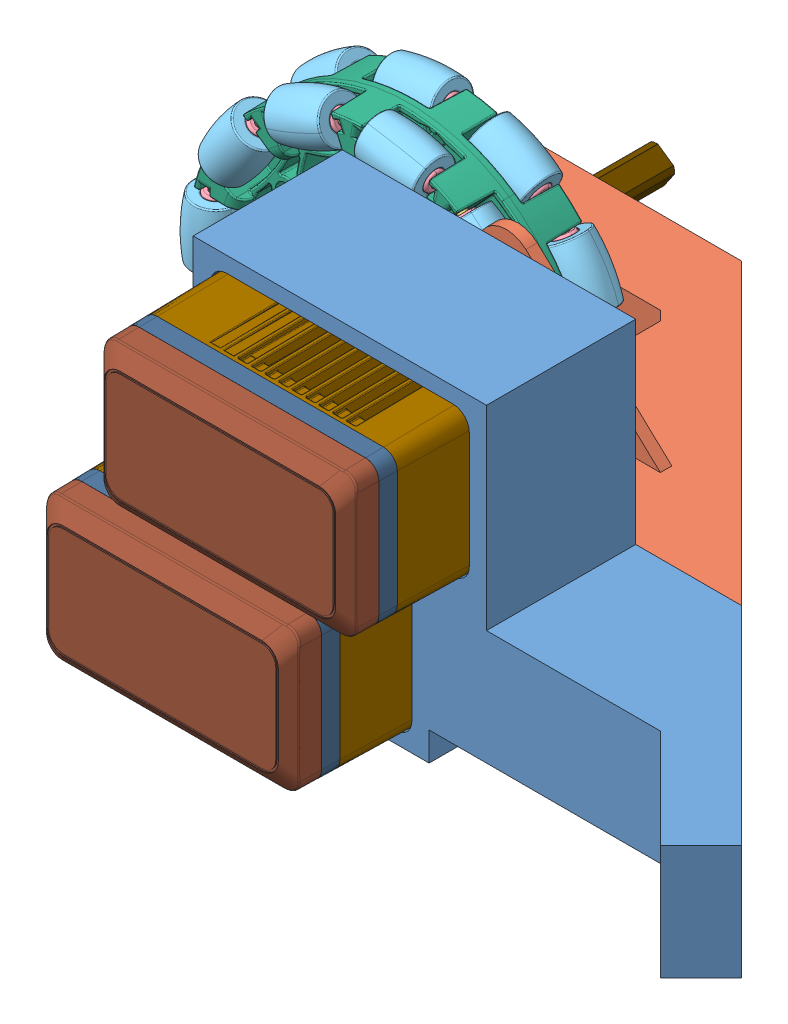
SolidWorks assembly Assem1, configuration Default. Lengths in mm.
Overall size (215.08 121.96 147.68).
139 component instances, 24 part files, 28 mates.
Components (placement in the parent):
- MotorBracket1-1: MotorBracket1 [Default] at (44.7562 139.8317 99.5148) size (165.36 74.93 54.97)
- V5 Smart Motor (276-4840) no cap 2-1: V5 Smart Motor (276-4840) no cap 2 [Default] at (82.8562 152.5317 238.3808) x (-1 0 0) z (0 0 -1) size (59.01 35.33 59.91)
  - 276-4840-900 Rev6_Instruction.step-1: 276-4840-900 Rev6_Instruction.step [Default] at (-14.3 0 -17.2) size (52.79 15.94 38.15)
    - 276-4840-901 Rev6.step-1: 276-4840-901 Rev6.step [Default] at (10.75 -10.05 17.8) x (-1 0 0) z (0 0 1) size (49.9 1.6 38.15)
    - 276-4840-902 Rev2.step-1: 276-4840-902 Rev2.step [Default] at (31.25 -9.25 6.2) x (0 0 -1) z (0 -1 0) size (10.35 11.39 15.94)
    - 276-4840-022 Rev4.step-1: 276-4840-022 Rev4.step [Default] at (31.25 -9.25 6.2) x (0 0 -1) z (1 0 0) size (10.26 9.1 5.51)
  - 276-4840-110 Rev10_Instruction.step-1: 276-4840-110 Rev10_Instruction.step [Default] at (12.7 0 14.7) size (35.33 35.33 31.1)
    - 276-4840-061 Rev7_Ring_Gear_Fixed01 .6 Rev3.step-1: 276-4840-061 Rev7_Ring_Gear_Fixed01 .6 Rev3.step [Default] at origin size (28.79 28.39 24.6)
    - 276-4840-018 Rev6.step-1: 276-4840-018 Rev6.step [Default] at (0 0 6.7) x (-0.483174 0.875524 0) z (0 0 1) size (26 26 12.3)
    - 276-4840-059 Rev2.step-1: 276-4840-059 Rev2.step [Default] at (0 0 10.3) size (28.4 28.4 8.5)
    - 276-4840-062 Rev1.step-1: 276-4840-062 Rev1.step [Default] at (-12.1353 8.8168 12.3) x (0.956835 -0.290632 0) z (-0.290632 -0.956835 0) size (3.2 6.56 3.2)
    - 276-4840-062 Rev1.step-2: 276-4840-062 Rev1.step [Default] at (12.1353 8.8168 12.3) x (0.978427 0.206591 0) z (0.206591 -0.978427 0) size (3.2 6.56 3.2)
    - 276-4840-062 Rev1.step-3: 276-4840-062 Rev1.step [Default] at (-12.1353 -8.8168 12.3) x (0.72563 0.688086 0) z (0.688086 -0.72563 0) size (3.2 6.56 3.2)
  - 276-4840-001 Rev38.step-1: 276-4840-001 Rev38.step [Default] at origin size (57.3 33 46.9)
  - 276-4840-005 Rev27.step-1: 276-4840-005 Rev27.step [Default] at (0 0 -17.95) size (56.17 31.87 12.9)
  - 276-4840-004 Rev16.step-1: 276-4840-004 Rev16.step [Default] at (0 0 -19.2) size (56.01 31.71 9.21)
  - 276-4840-009 Rev3.step-1: 276-4840-009 Rev3.step [Default] at (25.45 13.5 15.7) x (0.19987 -0.979823 0) z (-0.979823 -0.19987 0) size (3.4 41.31 4.34)
  - 276-4840-009 Rev3.step-2: 276-4840-009 Rev3.step [Default] at (-25.45 -13.5 15.7) x (-0.998855 0.047836 0) z (0.047836 0.998855 0) size (3.4 41.31 4.34)
  - 276-4840-009 Rev3.step-3: 276-4840-009 Rev3.step [Default] at (25.45 -13.5 15.7) x (-0.975374 0.220559 0) z (0.220559 0.975374 0) size (3.4 41.31 4.34)
  - 276-4840-009 Rev3.step-4: 276-4840-009 Rev3.step [Default] at (-25.45 13.5 15.7) x (-0.922256 0.38658 0) z (0.38658 0.922256 0) size (3.4 41.31 4.34)
  - 276-4840-025 Rev19.step-1: 276-4840-025 Rev19.step [Default] at (12.7 0 -22.63) x (-0.993315 0.115437 0) z (0 0 1) size (14.82 14.83 35.18)
- V5 Smart Motor (276-4840) no cap 2-2: V5 Smart Motor (276-4840) no cap 2 [Default] at (95.5562 188.4527 238.3808) x (-1 0 0) z (0 0 -1) size (59.01 35.33 59.91)
  - 276-4840-900 Rev6_Instruction.step-1: 276-4840-900 Rev6_Instruction.step [Default] at (-14.3 0 -17.2) size (52.79 15.94 38.15)
    - 276-4840-901 Rev6.step-1: 276-4840-901 Rev6.step [Default] at (10.75 -10.05 17.8) x (-1 0 0) z (0 0 1) size (49.9 1.6 38.15)
    - 276-4840-902 Rev2.step-1: 276-4840-902 Rev2.step [Default] at (31.25 -9.25 6.2) x (0 0 -1) z (0 -1 0) size (10.35 11.39 15.94)
    - 276-4840-022 Rev4.step-1: 276-4840-022 Rev4.step [Default] at (31.25 -9.25 6.2) x (0 0 -1) z (1 0 0) size (10.26 9.1 5.51)
  - 276-4840-110 Rev10_Instruction.step-1: 276-4840-110 Rev10_Instruction.step [Default] at (12.7 0 14.7) size (35.33 35.33 31.1)
    - 276-4840-061 Rev7_Ring_Gear_Fixed01 .6 Rev3.step-1: 276-4840-061 Rev7_Ring_Gear_Fixed01 .6 Rev3.step [Default] at origin size (28.79 28.39 24.6)
    - 276-4840-018 Rev6.step-1: 276-4840-018 Rev6.step [Default] at (0 0 6.7) x (-0.483174 0.875524 0) z (0 0 1) size (26 26 12.3)
    - 276-4840-059 Rev2.step-1: 276-4840-059 Rev2.step [Default] at (0 0 10.3) size (28.4 28.4 8.5)
    - 276-4840-062 Rev1.step-1: 276-4840-062 Rev1.step [Default] at (-12.1353 8.8168 12.3) x (0.956835 -0.290632 0) z (-0.290632 -0.956835 0) size (3.2 6.56 3.2)
    - 276-4840-062 Rev1.step-2: 276-4840-062 Rev1.step [Default] at (12.1353 8.8168 12.3) x (0.978427 0.206591 0) z (0.206591 -0.978427 0) size (3.2 6.56 3.2)
    - 276-4840-062 Rev1.step-3: 276-4840-062 Rev1.step [Default] at (-12.1353 -8.8168 12.3) x (0.72563 0.688086 0) z (0.688086 -0.72563 0) size (3.2 6.56 3.2)
  - 276-4840-001 Rev38.step-1: 276-4840-001 Rev38.step [Default] at origin size (57.3 33 46.9)
  - 276-4840-005 Rev27.step-1: 276-4840-005 Rev27.step [Default] at (0 0 -17.95) size (56.17 31.87 12.9)
  - 276-4840-004 Rev16.step-1: 276-4840-004 Rev16.step [Default] at (0 0 -19.2) size (56.01 31.71 9.21)
  - 276-4840-009 Rev3.step-1: 276-4840-009 Rev3.step [Default] at (25.45 13.5 15.7) x (0.19987 -0.979823 0) z (-0.979823 -0.19987 0) size (3.4 41.31 4.34)
  - 276-4840-009 Rev3.step-2: 276-4840-009 Rev3.step [Default] at (-25.45 -13.5 15.7) x (-0.998855 0.047836 0) z (0.047836 0.998855 0) size (3.4 41.31 4.34)
  - 276-4840-009 Rev3.step-3: 276-4840-009 Rev3.step [Default] at (25.45 -13.5 15.7) x (-0.975374 0.220559 0) z (0.220559 0.975374 0) size (3.4 41.31 4.34)
  - 276-4840-009 Rev3.step-4: 276-4840-009 Rev3.step [Default] at (-25.45 13.5 15.7) x (-0.922256 0.38658 0) z (0.38658 0.922256 0) size (3.4 41.31 4.34)
  - 276-4840-025 Rev19.step-1: 276-4840-025 Rev19.step [Default] at (12.7 0 -22.63) x (-0.993315 0.115437 0) z (0 0 1) size (14.82 14.83 35.18)
- 0.375_ ID x 0.875_ OD x 0.281_ WD (Radial Bearing) (217-3239)-1: 0.375_ ID x 0.875_ OD x 0.281_ WD (Radial Bearing) (217-3239) [Default] at (44.7562 152.5317 213.3576) x (0 0 -1) z (1 0 0) size (7.14 22.23 22.23)
- 0.375IDtoHSshaftInsert-1: 0.375IDtoHSshaftInsert [Default] at (44.7562 152.5317 213.3576) x (0.567741 0.823207 0) z (0 0 -1) size (9.53 9.53 5.54)
- 12T High Strength Metal Pinion with HS hole (276-2251)-1: 12T High Strength Metal Pinion with HS hole (276-2251) [Default] at (44.7562 152.5317 196.9048) x (0.567741 0.823207 0) z (0.823207 -0.567741 0) size (14.8 12.7 14.8)
- 36T Gear (276-2169-002).step-1: 36T Gear (276-2169-002).step [Default] at (70.1562 152.5317 194.4473) x (0.963194 -0.268806 0) z (0 0 1) size (40.08 40.08 9.53)
- 3.75_ High Strength Shaft (276-3524)-1: 3.75_ High Strength Shaft (276-3524) [Default] at (44.7562 152.5317 213.3576) x (-0.567741 -0.823207 0) z (0 0 -1) size (6.37 6.36 95.25)
- Holo_Motor_Shaft-1: Holo_Motor_Shaft [Default] at (70.1454 152.569 338.5008) x (0.875524 -0.483174 0) z (0 0 1) size (3.28 3.28 30.48)
- WheelBracket1-1: WheelBracket1 [Default] at (44.7562 139.8317 99.5148) size (119.38 54.97 66.04)
- 3.25_ Omni-Directional Wheel (276-3526) part-1: 3.25_ Omni-Directional Wheel (276-3526) part [Default] at (44.7562 152.5317 173.2048) x (0.567741 0.823207 0) z (0 0 1) size (90.82 89.11 34)
  - 3.25_ Omni-Directional Wheel (276-3526) .step-1: 3.25_ Omni-Directional Wheel (276-3526) .step [Default] at origin size (90.82 89.11 34)
    - Roller Assembly.step-1: Roller Assembly.step [Default] at (-0.0014 35.9575 7.1) x (0 0.963098 -0.269151) z (-1 0 0) size (14.05 14.05 18.75)
      - 276-3526-001 Rev 1.step-1: 276-3526-001 Rev 1.step [Default] at origin size (2 2 18.75)
      - 276-3526-003 Rev 1.step-1: 276-3526-003 Rev 1.step [Default] at origin size (6.15 6.15 14.2)
      - 276-3526-002 Rev 1.step-1: 276-3526-002 Rev 1.step [Default] x (0 0 1) z (-0.908956 0.416893 0) size (13.2 10.6 10.6)
    - Roller Assembly.step-2: Roller Assembly.step [Default] at (-19.4287 30.2567 7.1) x (0.421057 -0.655178 0.627258) z (-0.841254 -0.540641 0) size (14.05 14.05 18.75)
      - 276-3526-001 Rev 1.step-1: 276-3526-001 Rev 1.step [Default] at origin size (2 2 18.75)
      - 276-3526-003 Rev 1.step-1: 276-3526-003 Rev 1.step [Default] at origin size (6.15 6.15 14.2)
      - 276-3526-002 Rev 1.step-1: 276-3526-002 Rev 1.step [Default] x (0 0 1) z (-0.908956 0.416893 0) size (13.2 10.6 10.6)
    - Roller Assembly.step-3: Roller Assembly.step [Default] at (-35.5935 -5.1038 7.1) x (0.979746 0.140866 -0.142315) z (0.142315 -0.989821 0) size (14.05 14.05 18.75)
      - 276-3526-001 Rev 1.step-1: 276-3526-001 Rev 1.step [Default] at origin size (2 2 18.75)
      - 276-3526-003 Rev 1.step-1: 276-3526-003 Rev 1.step [Default] at origin size (6.15 6.15 14.2)
      - 276-3526-002 Rev 1.step-1: 276-3526-002 Rev 1.step [Default] x (0 0 1) z (-0.908956 0.416893 0) size (13.2 10.6 10.6)
    - Roller Assembly.step-4: Roller Assembly.step [Default] at (-10.1434 -34.4972 7.1) x (0.079373 0.27032 -0.959493) z (0.959493 -0.281733 0) size (14.05 14.05 18.75)
      - 276-3526-001 Rev 1.step-1: 276-3526-001 Rev 1.step [Default] at origin size (2 2 18.75)
      - 276-3526-003 Rev 1.step-1: 276-3526-003 Rev 1.step [Default] at origin size (6.15 6.15 14.2)
      - 276-3526-002 Rev 1.step-1: 276-3526-002 Rev 1.step [Default] x (0 0 1) z (-0.908956 0.416893 0) size (13.2 10.6 10.6)
    - Roller Assembly.step-5: Roller Assembly.step [Default] at (27.166 -23.5574 7.1) x (-0.355209 0.30779 -0.882662) z (0.654861 0.75575 0) size (14.05 14.05 18.75)
      - 276-3526-001 Rev 1.step-1: 276-3526-001 Rev 1.step [Default] at origin size (2 2 18.75)
      - 276-3526-003 Rev 1.step-1: 276-3526-003 Rev 1.step [Default] at origin size (6.15 6.15 14.2)
      - 276-3526-002 Rev 1.step-1: 276-3526-002 Rev 1.step [Default] x (0 0 1) z (-0.908956 0.416893 0) size (13.2 10.6 10.6)
    - Roller Assembly.step-6: Roller Assembly.step [Default] at (32.7138 14.9249 7.1) x (0.89908 0.410596 0.151875) z (-0.415415 0.909632 0) size (14.05 14.05 18.75)
      - 276-3526-001 Rev 1.step-1: 276-3526-001 Rev 1.step [Default] at origin size (2 2 18.75)
      - 276-3526-003 Rev 1.step-1: 276-3526-003 Rev 1.step [Default] at origin size (6.15 6.15 14.2)
      - 276-3526-002 Rev 1.step-1: 276-3526-002 Rev 1.step [Default] x (0 0 1) z (-0.908956 0.416893 0) size (13.2 10.6 10.6)
    - Roller Assembly.step-7: Roller Assembly.step [Default] at (19.4515 30.242 7.1) x (0.194707 0.302971 0.932898) z (-0.841254 0.540641 0) size (14.05 14.05 18.75)
      - 276-3526-001 Rev 1.step-1: 276-3526-001 Rev 1.step [Default] at origin size (2 2 18.75)
      - 276-3526-003 Rev 1.step-1: 276-3526-003 Rev 1.step [Default] at origin size (6.15 6.15 14.2)
      - 276-3526-002 Rev 1.step-1: 276-3526-002 Rev 1.step [Default] x (0 0 1) z (-0.908956 0.416893 0) size (13.2 10.6 10.6)
    - Roller Assembly.step-8: Roller Assembly.step [Default] at (-32.7025 14.9497 7.1) x (0.82743 -0.377875 0.415415) z (-0.415415 -0.909632 0) size (14.05 14.05 18.75)
      - 276-3526-001 Rev 1.step-1: 276-3526-001 Rev 1.step [Default] at origin size (2 2 18.75)
      - 276-3526-003 Rev 1.step-1: 276-3526-003 Rev 1.step [Default] at origin size (6.15 6.15 14.2)
      - 276-3526-002 Rev 1.step-1: 276-3526-002 Rev 1.step [Default] x (0 0 1) z (-0.908956 0.416893 0) size (13.2 10.6 10.6)
    - Roller Assembly.step-9: Roller Assembly.step [Default] at (-27.1838 -23.5369 7.1) x (0.578931 0.501646 -0.642799) z (0.654861 -0.75575 0) size (14.05 14.05 18.75)
      - 276-3526-001 Rev 1.step-1: 276-3526-001 Rev 1.step [Default] at origin size (2 2 18.75)
      - 276-3526-003 Rev 1.step-1: 276-3526-003 Rev 1.step [Default] at origin size (6.15 6.15 14.2)
      - 276-3526-002 Rev 1.step-1: 276-3526-002 Rev 1.step [Default] x (0 0 1) z (-0.908956 0.416893 0) size (13.2 10.6 10.6)
    - Roller Assembly.step-10: Roller Assembly.step [Default] at (10.1174 -34.5048 7.1) x (0.079373 -0.27032 -0.959493) z (0.959493 0.281733 0) size (14.05 14.05 18.75)
      - 276-3526-001 Rev 1.step-1: 276-3526-001 Rev 1.step [Default] at origin size (2 2 18.75)
      - 276-3526-003 Rev 1.step-1: 276-3526-003 Rev 1.step [Default] at origin size (6.15 6.15 14.2)
      - 276-3526-002 Rev 1.step-1: 276-3526-002 Rev 1.step [Default] x (0 0 1) z (-0.908956 0.416893 0) size (13.2 10.6 10.6)
    - Roller Assembly.step-11: Roller Assembly.step [Default] at (35.5896 -5.1307 7.1) x (0.988515 -0.142127 -0.05136) z (0.142315 0.989821 0) size (14.05 14.05 18.75)
      - 276-3526-001 Rev 1.step-1: 276-3526-001 Rev 1.step [Default] at origin size (2 2 18.75)
      - 276-3526-003 Rev 1.step-1: 276-3526-003 Rev 1.step [Default] at origin size (6.15 6.15 14.2)
      - 276-3526-002 Rev 1.step-1: 276-3526-002 Rev 1.step [Default] x (0 0 1) z (-0.908956 0.416893 0) size (13.2 10.6 10.6)
    - Roller Assembly.step-12: Roller Assembly.step [Default] at (10.1434 34.4972 -7.1) x (0.083119 0.283078 -0.955489) z (0.959493 -0.281733 0) size (14.05 14.05 18.75)
      - 276-3526-001 Rev 1.step-1: 276-3526-001 Rev 1.step [Default] at origin size (2 2 18.75)
      - 276-3526-003 Rev 1.step-1: 276-3526-003 Rev 1.step [Default] at origin size (6.15 6.15 14.2)
      - 276-3526-002 Rev 1.step-1: 276-3526-002 Rev 1.step [Default] x (0 0 1) z (-0.908956 0.416893 0) size (13.2 10.6 10.6)
    - Roller Assembly.step-13: Roller Assembly.step [Default] at (27.1838 23.5369 -7.1) x (0.582526 0.504762 -0.637086) z (0.654861 -0.75575 0) size (14.05 14.05 18.75)
      - 276-3526-001 Rev 1.step-1: 276-3526-001 Rev 1.step [Default] at origin size (2 2 18.75)
      - 276-3526-003 Rev 1.step-1: 276-3526-003 Rev 1.step [Default] at origin size (6.15 6.15 14.2)
      - 276-3526-002 Rev 1.step-1: 276-3526-002 Rev 1.step [Default] x (0 0 1) z (-0.908956 0.416893 0) size (13.2 10.6 10.6)
    - Roller Assembly.step-14: Roller Assembly.step [Default] at (35.5935 5.1038 -7.1) x (0.926341 0.133188 -0.352355) z (0.142315 -0.989821 0) size (14.05 14.05 18.75)
      - 276-3526-001 Rev 1.step-1: 276-3526-001 Rev 1.step [Default] at origin size (2 2 18.75)
      - 276-3526-003 Rev 1.step-1: 276-3526-003 Rev 1.step [Default] at origin size (6.15 6.15 14.2)
      - 276-3526-002 Rev 1.step-1: 276-3526-002 Rev 1.step [Default] x (0 0 1) z (-0.908956 0.416893 0) size (13.2 10.6 10.6)
    - Roller Assembly.step-15: Roller Assembly.step [Default] at (32.7025 -14.9497 -7.1) x (0.897398 -0.409828 0.163453) z (-0.415415 -0.909632 0) size (14.05 14.05 18.75)
      - 276-3526-001 Rev 1.step-1: 276-3526-001 Rev 1.step [Default] at origin size (2 2 18.75)
      - 276-3526-003 Rev 1.step-1: 276-3526-003 Rev 1.step [Default] at origin size (6.15 6.15 14.2)
      - 276-3526-002 Rev 1.step-1: 276-3526-002 Rev 1.step [Default] x (0 0 1) z (-0.908956 0.416893 0) size (13.2 10.6 10.6)
    - Roller Assembly.step-16: Roller Assembly.step [Default] at (19.4287 -30.2567 -7.1) x (0.277612 -0.431972 0.858098) z (-0.841254 -0.540641 0) size (14.05 14.05 18.75)
      - 276-3526-001 Rev 1.step-1: 276-3526-001 Rev 1.step [Default] at origin size (2 2 18.75)
      - 276-3526-003 Rev 1.step-1: 276-3526-003 Rev 1.step [Default] at origin size (6.15 6.15 14.2)
      - 276-3526-002 Rev 1.step-1: 276-3526-002 Rev 1.step [Default] x (0 0 1) z (-0.908956 0.416893 0) size (13.2 10.6 10.6)
    - Roller Assembly.step-17: Roller Assembly.step [Default] at (-0.0136 -35.9575 -7.1) x (0 -0.239919 0.970793) z (-1 0 0) size (14.05 14.05 18.75)
      - 276-3526-001 Rev 1.step-1: 276-3526-001 Rev 1.step [Default] at origin size (2 2 18.75)
      - 276-3526-003 Rev 1.step-1: 276-3526-003 Rev 1.step [Default] at origin size (6.15 6.15 14.2)
      - 276-3526-002 Rev 1.step-1: 276-3526-002 Rev 1.step [Default] x (0 0 1) z (-0.908956 0.416893 0) size (13.2 10.6 10.6)
    - Roller Assembly.step-18: Roller Assembly.step [Default] at (-19.4515 -30.242 -7.1) x (0.31008 0.482494 0.819176) z (-0.841254 0.540641 0) size (14.05 14.05 18.75)
      - 276-3526-001 Rev 1.step-1: 276-3526-001 Rev 1.step [Default] at origin size (2 2 18.75)
      - 276-3526-003 Rev 1.step-1: 276-3526-003 Rev 1.step [Default] at origin size (6.15 6.15 14.2)
      - 276-3526-002 Rev 1.step-1: 276-3526-002 Rev 1.step [Default] x (0 0 1) z (-0.908956 0.416893 0) size (13.2 10.6 10.6)
    - Roller Assembly.step-19: Roller Assembly.step [Default] at (-32.7138 -14.9249 -7.1) x (0.58758 0.268339 0.763377) z (-0.415415 0.909632 0) size (14.05 14.05 18.75)
      - 276-3526-001 Rev 1.step-1: 276-3526-001 Rev 1.step [Default] at origin size (2 2 18.75)
      - 276-3526-003 Rev 1.step-1: 276-3526-003 Rev 1.step [Default] at origin size (6.15 6.15 14.2)
      - 276-3526-002 Rev 1.step-1: 276-3526-002 Rev 1.step [Default] x (0 0 1) z (-0.908956 0.416893 0) size (13.2 10.6 10.6)
    - Roller Assembly.step-20: Roller Assembly.step [Default] at (-35.5896 5.1307 -7.1) x (0.965498 -0.138818 0.220323) z (0.142315 0.989821 0) size (14.05 14.05 18.75)
      - 276-3526-001 Rev 1.step-1: 276-3526-001 Rev 1.step [Default] at origin size (2 2 18.75)
      - 276-3526-003 Rev 1.step-1: 276-3526-003 Rev 1.step [Default] at origin size (6.15 6.15 14.2)
      - 276-3526-002 Rev 1.step-1: 276-3526-002 Rev 1.step [Default] x (0 0 1) z (-0.908956 0.416893 0) size (13.2 10.6 10.6)
    - Roller Assembly.step-21: Roller Assembly.step [Default] at (-27.166 23.5574 -7.1) x (0.75327 -0.652712 -0.080935) z (0.654861 0.75575 0) size (14.05 14.05 18.75)
      - 276-3526-001 Rev 1.step-1: 276-3526-001 Rev 1.step [Default] at origin size (2 2 18.75)
      - 276-3526-003 Rev 1.step-1: 276-3526-003 Rev 1.step [Default] at origin size (6.15 6.15 14.2)
      - 276-3526-002 Rev 1.step-1: 276-3526-002 Rev 1.step [Default] x (0 0 1) z (-0.908956 0.416893 0) size (13.2 10.6 10.6)
    - Roller Assembly.step-22: Roller Assembly.step [Default] at (-10.1174 34.5048 -7.1) x (0.123782 -0.421563 -0.898311) z (0.959493 0.281733 0) size (14.05 14.05 18.75)
      - 276-3526-001 Rev 1.step-1: 276-3526-001 Rev 1.step [Default] at origin size (2 2 18.75)
      - 276-3526-003 Rev 1.step-1: 276-3526-003 Rev 1.step [Default] at origin size (6.15 6.15 14.2)
      - 276-3526-002 Rev 1.step-1: 276-3526-002 Rev 1.step [Default] x (0 0 1) z (-0.908956 0.416893 0) size (13.2 10.6 10.6)
    - 276-3526-004 Rev 1.step-1: 276-3526-004 Rev 1.step [Default] at origin size (78.5 78.5 19.07)
Mates (geometry in assembly coordinates):
- Coincident1: coincident anti-aligned: plane of MotorBracket1-1 through (57.8062 165.4317 221.1808) normal (0 0 1); plane of V5 Smart Motor (276-4840) no cap 2-1/276-4840-001 Rev38.step-1 through (107.9062 165.4317 221.1808) normal (0 0 -1)
- Concentric1: concentric aligned: cylinder of MotorBracket1-1 through (107.9062 165.4317 221.1808) axis (0 0 1) radius 3.6; cone of V5 Smart Motor (276-4840) no cap 2-1/276-4840-001 Rev38.step-1 through (107.9062 165.4317 222.1808) axis (0 0 1)
- Concentric2: concentric aligned: cylinder of MotorBracket1-1 through (107.9062 139.6317 221.1808) axis (0 0 1) radius 3.6; cone of V5 Smart Motor (276-4840) no cap 2-1/276-4840-001 Rev38.step-1 through (107.9062 139.6317 222.1808) axis (0 0 1)
- Concentric4: concentric aligned: cylinder of MotorBracket1-1 through (120.6062 201.3527 221.1808) axis (0 0 1) radius 3.6; cone of V5 Smart Motor (276-4840) no cap 2-2/276-4840-001 Rev38.step-1 through (120.6062 201.3527 222.1808) axis (0 0 1)
- Concentric5: concentric aligned: cylinder of MotorBracket1-1 through (120.6062 175.5527 221.1808) axis (0 0 1) radius 3.6; cone of V5 Smart Motor (276-4840) no cap 2-2/276-4840-001 Rev38.step-1 through (120.6062 175.5527 222.1808) axis (0 0 1)
- Coincident3: coincident anti-aligned: plane of MotorBracket1-1 through (70.5062 201.3527 221.1808) normal (0 0 1); plane of V5 Smart Motor (276-4840) no cap 2-2/276-4840-001 Rev38.step-1 through (120.6062 201.3527 221.1808) normal (0 0 -1)
- Concentric6: concentric anti-aligned: cylinder of MotorBracket1-1 through (44.7562 152.5317 213.3576) axis (0 0 -1) radius 11.1125; cylinder of 0.375_ ID x 0.875_ OD x 0.281_ WD (Radial Bearing) (217-3239)-1 through (44.7562 152.5317 227.8946) axis (0 0 1) radius 11.113
- Coincident5: coincident anti-aligned: plane of MotorBracket1-1 through (44.7562 152.5317 213.3576) normal (0 0 -1); plane of 0.375_ ID x 0.875_ OD x 0.281_ WD (Radial Bearing) (217-3239)-1 through (44.7562 147.3687 213.3576) normal (0 0 1)
- Concentric7: concentric aligned: cylinder of 0.375_ ID x 0.875_ OD x 0.281_ WD (Radial Bearing) (217-3239)-1 through (44.7562 152.5317 227.8946) axis (0 0 1) radius 4.763; cylinder of 0.375IDtoHSshaftInsert-1 through (44.7562 152.5317 207.8204) axis (0 0 1) radius 4.7625
- Coincident6: coincident anti-aligned: plane of MotorBracket1-1 through (44.7562 152.5317 213.3576) normal (0 0 -1); plane of 0.375IDtoHSshaftInsert-1 through (44.7562 152.5317 213.3576) normal (0 0 1)
- Coincident7: coincident anti-aligned: plane of V5 Smart Motor (276-4840) no cap 2-1/276-4840-110 Rev10_Instruction.step-1/276-4840-018 Rev6.step-1 through (70.1562 152.5317 216.5808) normal (0 0 -1); plane of Holo_Motor_Shaft-1 through (70.1454 152.569 216.5808) normal (0 0 1)
- Coincident8: coincident anti-aligned: plane of V5 Smart Motor (276-4840) no cap 2-1/276-4840-110 Rev10_Instruction.step-1/276-4840-018 Rev6.step-1 through (72.3505 153.1653 211.3808) normal (-0.483174 -0.875524 0); plane of Holo_Motor_Shaft-1 through (69.5225 154.726 490.9008) normal (0.483174 0.875524 0)
- Coincident9: coincident anti-aligned: plane of V5 Smart Motor (276-4840) no cap 2-1/276-4840-110 Rev10_Instruction.step-1/276-4840-018 Rev6.step-1 through (67.9619 151.898 211.3808) normal (0.875524 -0.483174 0); plane of Holo_Motor_Shaft-1 through (67.9884 151.9462 490.9008) normal (-0.875524 0.483174 0)
- Concentric8: concentric anti-aligned: circle of V5 Smart Motor (276-4840) no cap 2-1/276-4840-110 Rev10_Instruction.step-1/276-4840-018 Rev6.step-1; circle of 36T Gear (276-2169-002).step-1
- Coincident10: coincident anti-aligned: plane of MotorBracket1-1 through (44.7562 152.5317 213.3576) normal (0 0 -1); plane of 3.75_ High Strength Shaft (276-3524)-1 through (44.7562 152.5317 213.3576) normal (0 0 1)
- Coincident11: coincident anti-aligned: plane of 0.375IDtoHSshaftInsert-1 through (48.7542 153.6312 207.8204) normal (-0.567741 -0.823207 0); plane of 3.75_ High Strength Shaft (276-3524)-1 through (44.825 156.3411 -91.4424) normal (0.567741 0.823207 0)
- Coincident12: coincident anti-aligned: plane of 0.375IDtoHSshaftInsert-1 through (40.6283 152.1388 207.8204) normal (0.823207 -0.567741 0); plane of 3.75_ High Strength Shaft (276-3524)-1 through (43.3382 156.068 -91.4424) normal (-0.823207 0.567741 0)
- Coincident13: coincident anti-aligned: plane of 12T High Strength Metal Pinion with HS hole (276-2251)-1 through (45.8557 148.5336 181.5746) normal (-0.823207 0.567741 0); plane of 3.75_ High Strength Shaft (276-3524)-1 through (48.5655 152.4628 -91.4424) normal (0.823207 -0.567741 0)
- Coincident14: coincident anti-aligned: plane of 12T High Strength Metal Pinion with HS hole (276-2251)-1 through (40.7581 151.4322 181.5746) normal (0.567741 0.823207 0); plane of 3.75_ High Strength Shaft (276-3524)-1 through (41.2199 151.1137 -91.4424) normal (-0.567741 -0.823207 0)
- Coincident15: coincident anti-aligned: plane of MotorBracket1-1 through (44.7562 165.2317 206.1948) normal (0 0 -1); plane of WheelBracket1-1 through (44.7562 165.2317 206.1948) normal (0 0 1)
- Coincident16: coincident aligned: plane of MotorBracket1-1 through (44.7562 165.2317 99.5148) normal (0 1 0); plane of WheelBracket1-1 through (44.7562 165.2317 99.5148) normal (0 1 0)
- Coincident17: coincident aligned: plane of MotorBracket1-1 through (44.7562 165.2317 99.5148) normal (0.707107 0 -0.707107); plane of WheelBracket1-1 through (44.7562 165.2317 99.5148) normal (0.707107 0 -0.707107)
- Coincident18: coincident anti-aligned: plane of 3.75_ High Strength Shaft (276-3524)-1 through (48.5655 152.4628 -91.4424) normal (0.823207 -0.567741 0); plane of 3.25_ Omni-Directional Wheel (276-3526) part-1/3.25_ Omni-Directional Wheel (276-3526) .step-1/276-3526-004 Rev 1.step-1 through (45.5673 148.1154 163.6798) normal (-0.823207 0.567741 0)
- Coincident19: coincident anti-aligned: plane of 3.75_ High Strength Shaft (276-3524)-1 through (41.2199 151.1137 -91.4424) normal (-0.567741 -0.823207 0); plane of 3.25_ Omni-Directional Wheel (276-3526) part-1/3.25_ Omni-Directional Wheel (276-3526) .step-1/276-3526-004 Rev 1.step-1 through (40.3399 151.7206 163.6798) normal (0.567741 0.823207 0)
- Distance1: distance = 14 mm anti-aligned: plane of 3.25_ Omni-Directional Wheel (276-3526) part-1/3.25_ Omni-Directional Wheel (276-3526) .step-1/276-3526-004 Rev 1.step-1 through (44.7562 152.5317 166.8548) normal (0 0 -1); plane of WheelBracket1-1 through (44.7562 165.2317 152.8548) normal (0 0 1)
- GearMate1: gear = 1 : 3 mm: cylinder of 36T Gear (276-2169-002).step-1 through (53.5416 160.0255 191.2723) axis (0 0 -1) radius 2.9504; cylinder of 12T High Strength Metal Pinion with HS hole (276-2251)-1 through (40.0536 156.4221 203.2548) axis (0 0 -1) radius 3
- Coincident21: coincident anti-aligned: plane of 36T Gear (276-2169-002).step-1 through (70.1562 152.5317 189.6848) normal (0 0 -1); plane of WheelBracket1-1 through (44.7562 165.2317 189.6848) normal (0 0 1)
- Distance2: distance = 11 mm anti-aligned: plane of 12T High Strength Metal Pinion with HS hole (276-2251)-1 through (47.6312 151.5088 190.5548) normal (0 0 -1); plane of 3.25_ Omni-Directional Wheel (276-3526) part-1/3.25_ Omni-Directional Wheel (276-3526) .step-1/276-3526-004 Rev 1.step-1 through (44.7562 152.5317 179.5548) normal (0 0 1)
